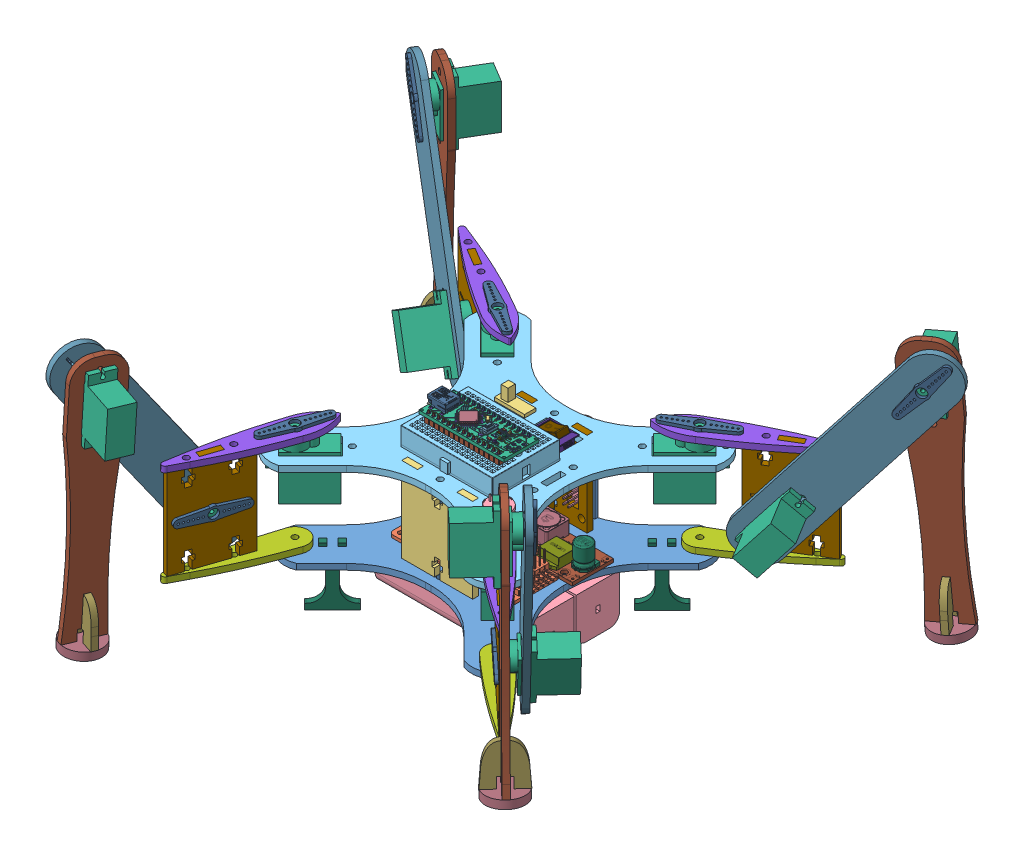
SolidWorks assembly SpiderBot_2_0, configuration Valor predeterminado. Lengths in mm.
Overall size (288.43 150.42 260.44).
147 component instances, 77 part files, 232 mates.
Components (placement in the parent):
- base-1: base [Valor predeterminado] at (7.4255 7.885 67) size (120.89 3 120.89)
- PCA9685-1: PCA9685 [Valor predeterminado] at (119.5232 12.385 80.9) size (67.25 16.5 25)
- suporte_mod-2: suporte_mod [Valor predeterminado] at (115.5232 50.885 96.5) size (36 46 3)
- Bateria-1: Bateria [Valor predeterminado] at (119.2732 7.885 80.5) x (-1 0 0) z (0 0 1) size (79 23 22)
- Bateria-3: Bateria [Valor predeterminado] at (119.2732 7.885 57.5) x (-1 0 0) z (0 0 1) size (79 23 22)
- Mini-Black.step-1: Mini-Black.step [Valor predeterminado] at (118.7863 59.6523 77.1335) size (48 9.4 35.7)
- Arduino_NANO_CH340.step-1: Arduino_NANO_CH340.step [Valor predeterminado] at (119.2913 68.1776 78.389) x (1 0 0) z (0 1 0) size (44.2 17.78 14.14)
  - Board_Geoms_6dc.step-1: Board_Geoms_6dc.step [Valor predeterminado] at origin size (44.2 17.78 2.36)
    - Pcb_6dc.step-1: Pcb_6dc.step [Valor predeterminado] at (-148.59 80.01 0) size (43.18 17.78 1.6)
    - topSilks_7595.step-1: topSilks_7595.step [Valor predeterminado] at (-148.59 80.01 0.07) size (44.2 13.15 0.15)
    - topTracks_6dc.step-1: topTracks_6dc.step [Valor predeterminado] at (-148.59 80.01 0.01) size (41.39 16.95 0.06)
    - botTracks_6dc.step-1: botTracks_6dc.step [Valor predeterminado] at (-148.59 80.01 -1.61) size (42.84 17.44 1.15)
  - Step_Models_6dc.step-1: Step_Models_6dc.step [Valor predeterminado] at origin size (41.36 17.78 14.14)
    - Top_6dc.step-1: Top_6dc.step [Valor predeterminado] at origin size (35.07 12.73 5)
      - J1_USB_Mini-B_Lumberg_2486_01_Horizontal_5F4AD4E6.step-1: J1_USB_Mini-B_Lumberg_2486_01_Horizontal_5F4AD4E6.step [Valor predeterminado] at (-16.51 0 0) x (0 -1 0) z (0 0 1) size (9.9 9.21 5)
      - R1_R_0603_1608Metric_5F4AD58B.step-1: R1_R_0603_1608Metric_5F4AD58B.step [Valor predeterminado] at (9.0425 3.81 0) size (1.6 0.8 0.45)
      - D1_LED_0603_1608Metric_5F4AD4A1.step-1: D1_LED_0603_1608Metric_5F4AD4A1.step [Valor predeterminado] at (11.9635 3.81 0) x (-1 0 0) z (0 0 1) size (1.6 0.8 1.1)
      - U1_TQFP_32_7x7mm_P08mm_5F4B89F1.step-1: U1_TQFP_32_7x7mm_P08mm_5F4B89F1.step [Valor predeterminado] at (-5.08 0 0) x (-0.707107 -0.707107 0) z (0 0 1) size (9 9 1.1)
      - SW1_SW_SPST_CK_RS282G05A3_5F4B980B.step-1: SW1_SW_SPST_CK_RS282G05A3_5F4B980B.step [Valor predeterminado] at (4.826 0.09 0) x (0 1 0) z (0 0 1) size (8 3.5 2.5)
      - D2_LED_0603_1608Metric_5F4BB16E.step-1: D2_LED_0603_1608Metric_5F4BB16E.step [Valor predeterminado] at (11.9635 1.27 0) x (-1 0 0) z (0 0 1) size (1.6 0.8 1.1)
      - D3_LED_0603_1608Metric_5F4BB181.step-1: D3_LED_0603_1608Metric_5F4BB181.step [Valor predeterminado] at (11.9635 -1.27 0) x (-1 0 0) z (0 0 1) size (1.6 0.8 1.1)
      - D4_LED_0603_1608Metric_5F4BB194.step-1: D4_LED_0603_1608Metric_5F4BB194.step [Valor predeterminado] at (11.9635 -3.81 0) x (-1 0 0) z (0 0 1) size (1.6 0.8 1.1)
      - R2_R_0603_1608Metric_5F4BB207.step-1: R2_R_0603_1608Metric_5F4BB207.step [Valor predeterminado] at (9.0425 1.27 0) size (1.6 0.8 0.45)
      - R3_R_0603_1608Metric_5F4BB218.step-1: R3_R_0603_1608Metric_5F4BB218.step [Valor predeterminado] at (9.0425 -1.27 0) size (1.6 0.8 0.45)
      - R4_R_0603_1608Metric_5F4BB229.step-1: R4_R_0603_1608Metric_5F4BB229.step [Valor predeterminado] at (9.0425 -3.81 0) size (1.6 0.8 0.45)
      - Y1_muRata_CSTxExxV_5F4BB25D.step-1: Y1_muRata_CSTxExxV_5F4BB25D.step [Valor predeterminado] at (0.254 4.318 0) x (0.707107 -0.707107 0) z (0 0 1) size (3.2 1.35 0.9)
    - Bot_6dc.step-1: Bot_6dc.step [Valor predeterminado] at origin size (39.62 17.78 11.54)
      - D5_D_0805_5F4AD4B4.step-1: D5_D_0805_5F4AD4B4.step [Valor predeterminado] at (-18.9715 3.556 -1.6) x (-1 0 0) z (0 0 -1) size (2 1.27 0.8)
      - U2_SOP_16_44x104mm_P127mm_5F4C8504.step-1: U2_SOP_16_44x104mm_P127mm_5F4C8504.step [Valor predeterminado] at (-9.53 0.356 -1.6) x (0 1 0) z (0 0 -1) size (6.4 10.4 2.1)
      - C1_C_0603_1608Metric_5F4BB0F2.step-1: C1_C_0603_1608Metric_5F4BB0F2.step [Valor predeterminado] at (-7.0865 -4.826 -1.6) x (-1 0 0) z (0 0 -1) size (1.6 0.8 0.8)
      - C2_C_0603_1608Metric_5F4BB0F3.step-1: C2_C_0603_1608Metric_5F4BB0F3.step [Valor predeterminado] at (-19.5325 -2.286 -1.6) x (-1 0 0) z (0 0 -1) size (1.6 0.8 0.8)
      - C4_C_0603_1608Metric_5F4BB124.step-1: C4_C_0603_1608Metric_5F4BB124.step [Valor predeterminado] at (9.1185 -4.064 -1.6) x (1 0 0) z (0 0 -1) size (1.6 0.8 0.8)
      - C5_C_0603_1608Metric_5F4BB135.step-1: C5_C_0603_1608Metric_5F4BB135.step [Valor predeterminado] at (10.6425 3.81 -1.6) x (1 0 0) z (0 0 -1) size (1.6 0.8 0.8)
      - J2_PinHeader_1x15_P254mm_Vertical_5F4BB1B7.step-1: J2_PinHeader_1x15_P254mm_Vertical_5F4BB1B7.step [Valor predeterminado] at (17.78 7.62 -1.6) x (0 1 0) z (0 0 -1) size (2.54 38.1 11.54)
      - J3_PinHeader_1x15_P254mm_Vertical_5F4BB1DA.step-1: J3_PinHeader_1x15_P254mm_Vertical_5F4BB1DA.step [Valor predeterminado] at (17.78 -7.62 -1.6) x (0 1 0) z (0 0 -1) size (2.54 38.1 11.54)
      - R5_R_0603_1608Metric_5F4BB23A.step-1: R5_R_0603_1608Metric_5F4BB23A.step [Valor predeterminado] at (-0.9905 -2.54 -1.6) x (-1 0 0) z (0 0 -1) size (1.6 0.8 0.45)
      - R6_R_0603_1608Metric_5F4BB24B.step-1: R6_R_0603_1608Metric_5F4BB24B.step [Valor predeterminado] at (-1.016 -4.318 -1.6) x (-1 0 0) z (0 0 -1) size (1.6 0.8 0.45)
      - R7_R_0603_1608Metric_5F4BB25C.step-1: R7_R_0603_1608Metric_5F4BB25C.step [Valor predeterminado] at (14.9605 3.81 -1.6) x (-1 0 0) z (0 0 -1) size (1.6 0.8 0.45)
      - Y2_muRata_CSTxExxV_5F4BB293.step-1: Y2_muRata_CSTxExxV_5F4BB293.step [Valor predeterminado] at (-13.462 -4.826 -1.6) x (-1 0 0) z (0 0 -1) size (3.2 1.35 0.9)
      - C6_CP_EIA_3216_18_Kemet_A_5F4BFB24.step-1: C6_CP_EIA_3216_18_Kemet_A_5F4BFB24.step [Valor predeterminado] at (-18.97 0 -1.6) x (-1 0 0) z (0 0 -1) size (3.2 1.6 1.8)
      - C7_CP_EIA_3216_18_Kemet_A_5F4BFB36.step-1: C7_CP_EIA_3216_18_Kemet_A_5F4BFB36.step [Valor predeterminado] at (12.62 1.27 -1.6) x (-1 0 0) z (0 0 -1) size (3.2 1.6 1.8)
      - U3_SOT_89_3_5F4BFB48.step-1: U3_SOT_89_3_5F4BFB48.step [Valor predeterminado] at (12.7 -2.54 -1.6) x (-1 0 0) z (0 0 -1) size (4 4.5 1.52)
- Camera OV7670.STEP-1: Camera OV7670.STEP [Valor predeterminado] at (119.0232 31.335 36.768) x (0 -1 0) z (0 0 -1) size (34 35 28.6)
  - PcbForCamera.STEP-1: PcbForCamera.STEP [Valor predeterminado] at origin size (34 35 1.5)
  - CameraLens.STEP-1: CameraLens.STEP [Valor predeterminado] at (0 4.5 1.5) size (24 17.5 18.5)
  - pan head cross recess screw_iso_ISO 7045 - M1.6 x 6 - Z - 6N.STEP-1: pan head cross recess screw_iso_ISO 7045 - M1.6 x 6 - Z - 6N.STEP [Valor predeterminado] at (-10 4.5 -1.3) x (0 0 1) z (-0.934163 -0.356846 0) size (7.27 3.2 3.2)
  - pan head cross recess screw_iso_ISO 7045 - M1.6 x 6 - Z - 6N.STEP-2: pan head cross recess screw_iso_ISO 7045 - M1.6 x 6 - Z - 6N.STEP [Valor predeterminado] at (10 4.5 -1.3) x (0 0 1) z (-0.934163 -0.356846 0) size (7.27 3.2 3.2)
  - PLS (DS1021-2xN)_DS1021-2x9.STEP-1: PLS (DS1021-2xN)_DS1021-2x9.STEP [Valor predeterminado] at (-10.16 -10.96 -2.5) size (22.86 5.08 11.6)
  - CAP 1206___ _________.STEP-1: CAP 1206___ _________.STEP [Valor predeterminado] at (12.3944 -3.3656 -0.812) size (3.2 1.62 1.62)
  - CAP 1206___ _________.STEP-2: CAP 1206___ _________.STEP [Valor predeterminado] at (8.833 13.1436 -0.812) size (3.2 1.62 1.62)
  - CAP 1206___ _________.STEP-3: CAP 1206___ _________.STEP [Valor predeterminado] at (-4.7413 13.3527 -0.812) size (3.2 1.62 1.62)
  - CAP 1206___ _________.STEP-4: CAP 1206___ _________.STEP [Valor predeterminado] at (-12.2243 8.8938 -0.812) size (3.2 1.62 1.62)
  - CAP 1206___ _________.STEP-5: CAP 1206___ _________.STEP [Valor predeterminado] at (-11.8299 -3.7667 -0.812) size (3.2 1.62 1.62)
  - CAP 0603___ _________.STEP-1: CAP 0603___ _________.STEP [Valor predeterminado] at (13.1952 -0.5568 -0.412) size (1.6 0.82 0.82)
  - CAP 0603___ _________.STEP-2: CAP 0603___ _________.STEP [Valor predeterminado] at (14.6505 6.2818 -0.412) size (1.6 0.82 0.82)
  - CAP 0603___ _________.STEP-3: CAP 0603___ _________.STEP [Valor predeterminado] at (8.112 11.3604 -0.412) size (1.6 0.82 0.82)
  - CAP 0603___ _________.STEP-4: CAP 0603___ _________.STEP [Valor predeterminado] at (-14.0856 5.7012 -0.412) size (1.6 0.82 0.82)
  - CAP 0603___ _________.STEP-5: CAP 0603___ _________.STEP [Valor predeterminado] at (-13.8777 -1.2547 -0.412) size (1.6 0.82 0.82)
  - CAP 0603___ _________.STEP-6: CAP 0603___ _________.STEP [Valor predeterminado] at (9.9936 -5.5766 -0.412) x (0 -1 0) z (0 0 1) size (1.6 0.82 0.82)
  - Stackpole CSR0402 Res___ _________.STEP-1: Stackpole CSR0402 Res___ _________.STEP [Valor predeterminado] at (2.2276 13.9111 0) x (0 -1 0) z (1 0 0) size (0.5 0.32 1.05)
  - Stackpole CSR0402 Res___ _________.STEP-2: Stackpole CSR0402 Res___ _________.STEP [Valor predeterminado] at (-9.8479 14.1877 0) x (0 -1 0) z (1 0 0) size (0.5 0.32 1.05)
  - SC-70-5___ _________.STEP-1: SC-70-5___ _________.STEP [Valor predeterminado] at (14.6025 3.5126 0) x (1 0 0) z (0 1 0) size (2 1.1 2.12)
  - SC-70-5___ _________.STEP-2: SC-70-5___ _________.STEP [Valor predeterminado] at (-14.2433 2.7104 0) x (-1 0 0) z (0 -1 0) size (2 1.1 2.12)
  - Stackpole CSR0402 Res___ _________.STEP-3: Stackpole CSR0402 Res___ _________.STEP [Valor predeterminado] at (-10.4133 -5.8042 0) x (-1 0 0) z (0 -1 0) size (0.5 0.32 1.05)
- suporte_mod_cam-1: suporte_mod_cam [Valor predeterminado] at (123.0232 10.885 38.5) x (-1 0 0) z (0 0 1) size (36 46 3)
- UBEC_certo-1: UBEC_certo [Valor predeterminado] at (100.2806 26.8872 90.152) size (44 18 7.45)
- LM2596 DC-DC StepDown Converter v1.step-1: LM2596 DC-DC StepDown Converter v1.step [Valor predeterminado] at (113.7732 22.2177 57.2327) x (-1 0 0) z (0 1 0) size (43 21 14.15)
  - Board v5.step-1: Board v5.step [Valor predeterminado] at (0 -9.7327 -11.3327) x (1 0 0) z (0 -1 0) size (43 1.7 21)
  - Trimpot 3296W v1.step-1: Trimpot 3296W v1.step [Valor predeterminado] at (-14.54 7.2723 -9.7327) x (-1 0 0) z (0 0 1) size (9.56 4.83 14.15)
  - CDRH127_470M v1.step-1: CDRH127_470M v1.step [Valor predeterminado] at (-15.855 -2.8827 -9.7427) x (0 -1 0) z (0 0 1) size (12.76 12.29 7.41)
  - CAPSMD220-35 v1.step-1: CAPSMD220-35 v1.step [Valor predeterminado] at (-4.2601 1.0246 -9.7327) x (0 1 0) z (0 0 1) size (9 8.3 10.7)
  - CAPSMD100-50 v1.step-1: CAPSMD100-50 v1.step [Valor predeterminado] at (-38.35 0.7473 -9.7327) x (0 1 0) z (0 0 1) size (9 8.3 10.7)
  - TO-263BA v2.step-1: TO-263BA v2.step [Valor predeterminado] at (-31.9 -3.4327 -9.7327) size (10.64 15.85 4.81)
  - DO-214AC-DIOM5127X23N v1.step-1: DO-214AC-DIOM5127X23N v1.step [Valor predeterminado] at (-32.735 -7.9827 -9.7327) size (5.3 2.8 2.3)
  - Resistor 0603 v1.step-1: Resistor 0603 v1.step [Valor predeterminado] at (-19.95 10.2673 -9.7327) x (0 -1 0) z (-1 0 0) size (2.1 0.6 0.8)
  - Resistor 0603 v1 (1).step-1: Resistor 0603 v1 (1).step [Valor predeterminado] at (-6.75 9.7673 -9.7327) x (0 -1 0) z (-1 0 0) size (2.1 0.6 0.8)
  - CAP0603 v1.step-1: CAP0603 v1.step [Valor predeterminado] at (-21.085 5.9823 -9.7327) x (0 -1 0) z (0 0 1) size (1.61 0.81 0.31)
  - FCrth 150060BS55040 v1.step-1: FCrth 150060BS55040 v1.step [Valor predeterminado] at (-5.89 8.9773 -9.7327) x (0 -1 0) z (0 0 1) size (1.6 0.8 0.4)
  - CAP0603 v1 (1).step-1: CAP0603 v1 (1).step [Valor predeterminado] at (-35.385 -5.5177 -9.7327) x (0 -1 0) z (0 0 1) size (1.61 0.81 0.31)
- base_cima-1: base_cima [Valor predeterminado] at (7.4255 50.885 67) size (128.99 3 128.99)
- Servo-1: Servo [Valor predeterminado] at (59.6659 32.485 17.5951) x (0.707107 0 0.707107) z (-0.707107 0 0.707107) size (31.9 29.9 11.8)
- Servo-2: Servo [Valor predeterminado] at (170.5367 32.485 9.2513) x (-0.707107 0 0.707107) z (-0.707107 0 -0.707107) size (31.9 29.9 11.8)
- Servo-3: Servo [Valor predeterminado] at (178.6684 32.485 119.9099) x (-0.707107 0 -0.707107) z (0.707107 0 -0.707107) size (31.9 29.9 11.8)
- Servo-4: Servo [Valor predeterminado] at (67.8684 32.485 128.6073) x (0.707107 0 -0.707107) z (0.707107 0 0.707107) size (31.9 29.9 11.8)
- Perna_baciadown-1: Perna_baciadown [Valor predeterminado] at (183.5595 10.885 132.1762) x (0.67976 0 -0.733435) z (0.733435 0 0.67976) size (13 3 60.1)
- Perna_baciaup-1: Perna_baciaup [Valor predeterminado] at (170.444 59.485 119.9618) x (0.67976 0 -0.733435) z (0.733435 0 0.67976) size (13.12 3 71.83)
- Perna_coxa-1: Perna_coxa [Valor predeterminado] at (196.281 36.385 141.9216) x (0 1 0) z (0.733435 0 0.67976) size (51.6 3 36)
- Servo_knob2-1: Servo_knob2 [Valor predeterminado] at (170.3246 59.185 119.9099) x (-0.727643 0 -0.685956) z (0.685956 0 -0.727643) size (32.4 4.8 6.6)
- Servo-6: Servo [Valor predeterminado] at (212.0513 44.249 119.7247) x (-0.251237 -0.9395 -0.232851) z (-0.689062 0.342549 -0.638634) size (31.9 29.9 11.8)
- Servo_knob2-3: Servo_knob2 [Valor predeterminado] at (196.4849 36.685 141.7016) x (0.733432 -0.00261 0.679757) z (-0.001914 -0.999997 -0.001774) size (32.4 4.8 6.6)
- Pé_com_antiderrapante-1: Pé_com_antiderrapante [Valor predeterminado] at (215.1821 130.5825 159.4395) x (0.729921 0.097767 0.676503) z (-0.67976 0 0.733435) size (24 122.6 3)
- comp_pé-1: comp_pé [Valor predeterminado] at (230.6854 6.2285 162.9006) x (-0.67976 0 0.733435) z (-0.729921 -0.097767 -0.676503) size (19 20 3)
- Antiderrapante-1: Antiderrapante [Valor predeterminado] at (223.4327 2.1038 169.1472) x (0.729921 0.097767 0.676503) z (-0.67976 0 0.733435) size (19 4 19)
- Canela_mod-1: Canela_mod [Valor predeterminado] at (219.7108 109.8107 156.0015) x (0.689062 -0.342549 0.638634) z (0.251237 0.9395 0.232851) size (24 3 124.6)
- Servo_knob2-4: Servo_knob2 [Valor predeterminado] at (220.1772 112.2805 156.8427) x (-0.247031 -0.941571 -0.228953) z (0.690581 -0.336814 0.640042) size (32.4 4.8 6.6)
- Servo-7: Servo [Valor predeterminado] at (205.9111 118.729 180.0247) x (0.071706 -0.995209 0.066458) z (0.729921 0.097767 0.676503) size (31.9 29.9 11.8)
- Perna_baciaup-2: Perna_baciaup [Valor predeterminado] at (67.8822 59.485 17.5691) x (-0.51295 0 0.858418) z (-0.858418 0 -0.51295) size (13.12 3 71.83)
- Servo_knob2-8: Servo_knob2 [Valor predeterminado] at (68.0098 59.185 17.5951) x (0.851179 0 0.524875) z (-0.524875 0 0.851179) size (32.4 4.8 6.6)
- Servo_knob2-9: Servo_knob2 [Valor predeterminado] at (-3.6674 103.1368 -17.3143) x (0.479294 -0.829608 0.286404) z (-0.712151 -0.558346 -0.425548) size (32.4 4.8 6.6)
- Servo-11: Servo [Valor predeterminado] at (4.9713 109.0457 -43.2559) x (-0.001293 -0.999999 -0.000773) z (-0.858417 0.001507 -0.51295) size (31.9 29.9 11.8)
- Pé_com_antiderrapante-3: Pé_com_antiderrapante [Valor predeterminado] at (-0.8391 121.5366 -21.7984) x (-0.858417 0.001507 -0.51295) z (0.51295 0 -0.858418) size (24 122.6 3)
- comp_pé-3: comp_pé [Valor predeterminado] at (-6.3922 -3.561 -15.7971) x (0.51295 0 -0.858418) z (0.858417 -0.001507 0.51295) size (19 20 3)
- Antiderrapante-3: Antiderrapante [Valor predeterminado] at (-0.2553 -7.5632 -23.2104) x (-0.858417 0.001507 -0.51295) z (0.51295 0 -0.858418) size (19 4 19)
- Canela_mod-3: Canela_mod [Valor predeterminado] at (-2.5388 100.9682 -16.2903) x (-0.709215 -0.563394 -0.423794) z (-0.483627 0.826189 -0.288993) size (24 3 124.6)
- Servo-12: Servo [Valor predeterminado] at (25.5355 44.8835 25.4151) x (0.483627 -0.826189 0.288993) z (0.709215 0.563394 0.423794) size (31.9 29.9 11.8)
- Servo_knob2-10: Servo_knob2 [Valor predeterminado] at (37.9003 36.685 1.7) x (-0.858415 -0.00261 -0.512949) z (0.00224 -0.999997 0.001339) size (32.4 4.8 6.6)
- Perna_baciadown-3: Perna_baciadown [Valor predeterminado] at (52.5195 10.885 8.3389) x (-0.51295 0 0.858418) z (-0.858418 0 -0.51295) size (13 3 60.1)
- Perna_coxa-3: Perna_coxa [Valor predeterminado] at (38.0541 36.385 1.4424) x (0 1 0) z (-0.858418 0 -0.51295) size (51.6 3 36)
- Perna_coxa-4: Perna_coxa [Valor predeterminado] at (58.5011 36.385 152.982) x (0 1 0) z (-0.317345 0 0.94831) size (51.6 3 36)
- Servo_knob2-11: Servo_knob2 [Valor predeterminado] at (55.3717 36.685 151.9348) x (-0.317345 0.000085 0.94831) z (0.000027 1 -0.000081) size (32.4 4.8 6.6)
- Servo_knob2-12: Servo_knob2 [Valor predeterminado] at (67.8684 59.185 120.2635) x (0.325377 0 -0.945584) z (0.945584 0 0.325377) size (32.4 4.8 6.6)
- Perna_baciaup-3: Perna_baciaup [Valor predeterminado] at (67.8703 59.485 120.3937) x (0.94831 0 0.317345) z (-0.317345 0 0.94831) size (13.12 3 71.83)
- Perna_baciadown-4: Perna_baciadown [Valor predeterminado] at (62.1418 10.885 137.3758) x (0.94831 0 0.317345) z (-0.317345 0 0.94831) size (13 3 60.1)
- Servo_knob2-13: Servo_knob2 [Valor predeterminado] at (36.2364 103.1908 193.3603) x (0.180723 -0.822001 -0.540049) z (0.260858 0.569485 -0.779512) size (32.4 4.8 6.6)
- Servo-13: Servo [Valor predeterminado] at (63.5241 108.7739 195.9531) x (-0.016613 -0.998629 0.049644) z (0.31691 -0.05235 -0.94701) size (31.9 29.9 11.8)
- Pé_com_antiderrapante-4: Pé_com_antiderrapante [Valor predeterminado] at (41.5364 121.5708 194.2235) x (0.31691 -0.05235 -0.94701) z (0.94831 0 0.317345) size (24 122.6 3)
- comp_pé-4: comp_pé [Valor predeterminado] at (32.3471 -3.4362 196.4746) x (0.94831 0 0.317345) z (-0.31691 0.05235 0.94701) size (19 20 3)
- Antiderrapante-4: Antiderrapante [Valor predeterminado] at (40.8343 -7.3537 201.0851) x (0.31691 -0.05235 -0.94701) z (0.94831 0 0.317345) size (19 4 19)
- Canela_mod-4: Canela_mod [Valor predeterminado] at (36.4203 101.0099 191.8654) x (0.261955 0.564463 -0.782791) z (-0.179129 0.825458 0.535286) size (24 3 124.6)
- Servo-14: Servo [Valor predeterminado] at (27.4494 38.2248 151.2383) x (0.179129 -0.825458 -0.535286) z (-0.261955 -0.564463 0.782791) size (31.9 29.9 11.8)
- Servo-16: Servo [Valor predeterminado] at (227.1986 104.6122 -40.1648) x (0.063997 -0.997191 -0.038929) z (-0.851949 -0.074907 0.518239) size (31.9 29.9 11.8)
- Servo-17: Servo [Valor predeterminado] at (221.4875 37.5346 19.9606) x (-0.539458 -0.775437 0.328151) z (0.662494 -0.631425 -0.402994) size (31.9 29.9 11.8)
- Canela_mod-6: Canela_mod [Valor predeterminado] at (245.2223 97.1208 -19.5256) x (-0.662494 0.631425 0.402994) z (0.539458 0.775437 -0.328151) size (24 3 124.6)
- comp_pé-6: comp_pé [Valor predeterminado] at (253.5176 -7.3343 -21.7624) x (-0.519699 0 -0.85435) z (0.851949 0.074907 -0.518239) size (19 20 3)
- Pé_com_antiderrapante-6: Pé_com_antiderrapante [Valor predeterminado] at (242.6319 117.5265 -24.5045) x (-0.851949 -0.074907 0.518239) z (-0.519699 0 -0.85435) size (24 122.6 3)
- Servo_knob2-17: Servo_knob2 [Valor predeterminado] at (200.52 36.685 1.4632) x (0.85435 0.000085 -0.519699) z (-0.000073 1 0.000044) size (32.4 4.8 6.6)
- Servo_knob2-18: Servo_knob2 [Valor predeterminado] at (246.4787 99.1708 -20.6409) x (-0.543487 -0.771572 0.330602) z (-0.659192 0.636142 0.400985) size (32.4 4.8 6.6)
- Servo_knob2-19: Servo_knob2 [Valor predeterminado] at (170.5367 59.185 17.5951) x (-0.858727 0 0.512434) z (-0.512434 0 -0.858727) size (32.4 4.8 6.6)
- Perna_baciadown-6: Perna_baciadown [Valor predeterminado] at (185.9535 10.885 8.2171) x (-0.519699 0 -0.85435) z (0.85435 0 -0.519699) size (13 3 60.1)
- Perna_baciaup-5: Perna_baciaup [Valor predeterminado] at (170.6193 59.485 17.4944) x (-0.519699 0 -0.85435) z (0.85435 0 -0.519699) size (13.12 3 71.83)
- Perna_coxa-6: Perna_coxa [Valor predeterminado] at (198.805 36.385 -1.3562) x (0 1 0) z (0.85435 0 -0.519699) size (51.6 3 36)
- suporte_embaixo-1: suporte_embaixo [Valor predeterminado] at (74.9476 7.885 22.6787) x (0.707107 0 0.707107) z (-0.707107 0 0.707107) size (20 29.5 3)
- suporte_embaixo-2: suporte_embaixo [Valor predeterminado] at (156.5279 7.885 29.7498) x (0.707107 0 -0.707107) z (0.707107 0 0.707107) size (20 29.5 3)
- suporte_embaixo-3: suporte_embaixo [Valor predeterminado] at (158.6492 7.885 106.1289) x (0.707107 0 0.707107) z (-0.707107 0 0.707107) size (20 29.5 3)
- suporte_embaixo-4: suporte_embaixo [Valor predeterminado] at (82.0186 7.885 108.2502) x (-0.707107 0 0.707107) z (-0.707107 0 -0.707107) size (20 29.5 3)
- Placa_GY521-1: Placa_GY521 [Predeterminado] at (118.6183 50.885 67.7208) x (0.007037 0 -0.999975) z (-0.999975 0 -0.007037) size (20.27 65.96 16.25)
- KCD1-11-2P-Off.step-1: KCD1-11-2P-Off.step [Valor predeterminado] at (128.815 54.751 49.6928) x (0 0 -1) z (1 0 0) size (10.5 19.01 15.2)
  - eBom-prt0.step-1: eBom-prt0.step [Valor predeterminado] at origin size (10.5 16.7 15.2)
  - eBom-prt1.step-1: eBom-prt1.step [Valor predeterminado] at (0 -0.9 0) x (1 0 0) z (0 0.228555 0.973531) size (7.4 7.35 10.6)
  - eBom-prt2.step-1: eBom-prt2.step [Valor predeterminado] at (0 -4.8504 0.3584) x (1 0 0) z (0 -0.285651 0.958334) size (5.24 1.4 9.6)
  - eBom-prt3.step-1: eBom-prt3.step [Valor predeterminado] at (0 0.1321 -0.2423) x (1 0 0) z (0 0.228555 0.973531) size (2.38 6.89 2.38)
- switch_pequeno-1: switch_pequeno [Valor predeterminado] at (98.5232 55.5004 49.8053) size (15.35 16.5 5.75)
- Buzzer_Active.stp-1: Buzzer_Active.stp [Valor predeterminado] at (145.1358 57.9073 98.5749) x (0.989214 0 -0.146479) z (0 -1 0) size (11.85 11.85 12.2)
- LED-1: LED [Default] at (88.3285 7.585 43.1958) x (0 0 -1) z (-1 0 0) size (5.5 35.6 6)
- LED-2: LED [Default] at (94.5547 7.585 43.1958) x (-0.444848 0 -0.895606) z (-0.895606 0 0.444848) size (5.5 35.6 6)
- Antiderrapante-7: Antiderrapante [Valor predeterminado] at (249.9458 -11.2257 -30.7055) x (-0.903442 -0.074462 0.422195) z (-0.423908 0.008151 -0.905669) size (19 4 19)
- Harness_1-SpiderBot_2_0-1: Harness_1-SpiderBot_2_0 [Valor predeterminado] at origin
Mates (geometry in assembly coordinates):
- Bloquear1: lock: unknown of Mini-Black.step-1; unknown of Arduino_NANO_CH340.step-1/Board_Geoms_6dc.step-1/Pcb_6dc.step-1
- Coincidente34: coincident anti-aligned: plane of base-1 through (7.4255 10.885 38.5) normal (0 0 1); plane of suporte_mod_cam-1 through (123.0232 10.885 38.5) normal (0 0 -1)
- Coincidente35: coincident anti-aligned: plane of base-1 through (101.2732 10.885 67) normal (1 0 0); plane of suporte_mod_cam-1 through (101.2732 8.885 41.5) normal (-1 0 0)
- Coincidente39: coincident anti-aligned: plane of base-1 through (7.4255 10.885 67) normal (0 1 0); plane of suporte_mod_cam-1 through (120.7732 10.885 41.5) normal (0 -1 0)
- Coincidente40: coincident anti-aligned: plane of base-1 through (137.2732 10.885 67) normal (-1 0 0); plane of suporte_mod-2 through (137.2732 52.885 99.5) normal (1 0 0)
- Coincidente41: coincident anti-aligned: plane of base-1 through (7.4255 10.885 96.5) normal (0 0 1); plane of suporte_mod-2 through (115.5232 50.885 96.5) normal (0 0 -1)
- Coincidente42: coincident anti-aligned: plane of base-1 through (7.4255 10.885 67) normal (0 1 0); plane of suporte_mod-2 through (120.7732 10.885 99.5) normal (0 -1 0)
- Paralelo3: parallel anti-aligned: plane of Camera OV7670.STEP-1/PcbForCamera.STEP-1 through (119.0232 31.335 36.768) normal (0 0 1); plane of suporte_mod_cam-1 through (123.0232 10.885 38.5) normal (0 0 -1)
- Concêntrico2: concentric anti-aligned: circle of Camera OV7670.STEP-1/PcbForCamera.STEP-1; circle of suporte_mod_cam-1
- Paralelo4: parallel aligned: plane of Camera OV7670.STEP-1/PcbForCamera.STEP-1 through (136.5232 14.335 35.268) normal (1 0 0); plane of suporte_mod_cam-1 through (137.2732 52.885 41.5) normal (1 0 0)
- Coincidente43: coincident anti-aligned: plane of suporte_mod_cam-1 through (123.0232 10.885 41.5) normal (0 0 1); plane of base_cima-1 through (7.4255 53.885 41.5) normal (0 0 -1)
- Coincidente44: coincident anti-aligned: plane of suporte_mod_cam-1 through (137.2732 52.885 41.5) normal (1 0 0); plane of base_cima-1 through (137.2732 53.885 67) normal (-1 0 0)
- Coincidente45: coincident anti-aligned: plane of suporte_mod_cam-1 through (120.7732 50.885 41.5) normal (0 1 0); plane of base_cima-1 through (7.4255 50.885 67) normal (0 -1 0)
- Coincidente46: coincident anti-aligned: plane of base_cima-1 through (66.592 53.885 7.8335) normal (-0.707107 0 0.707107); plane of Servo-1 through (83.9197 55.185 25.1612) normal (0.707107 0 -0.707107)
- Coincidente47: coincident anti-aligned: plane of base_cima-1 through (8.8433 53.885 68.4178) normal (0.707107 0 0.707107); plane of Servo-1 through (68.0098 55.185 9.2513) normal (-0.707107 0 -0.707107)
- Coincidente48: coincident anti-aligned: plane of base_cima-1 through (7.4255 50.885 67) normal (0 -1 0); plane of Servo-1 through (56.3425 50.885 14.2717) normal (0 1 0)
- Coincidente49: coincident anti-aligned: plane of base_cima-1 through (6.8433 53.885 67.5822) normal (0.707107 0 -0.707107); plane of Servo-4 through (59.5245 55.185 120.2635) normal (-0.707107 0 0.707107)
- Coincidente50: coincident anti-aligned: plane of base_cima-1 through (60.1067 53.885 119.6813) normal (0.707107 0 0.707107); plane of Servo-4 through (75.4344 55.185 104.3536) normal (-0.707107 0 -0.707107)
- Coincidente51: coincident anti-aligned: plane of base_cima-1 through (7.4255 50.885 67) normal (0 -1 0); plane of Servo-4 through (64.545 50.885 131.9307) normal (0 1 0)
- Coincidente54: coincident anti-aligned: plane of base_cima-1 through (7.4255 50.885 67) normal (0 -1 0); plane of Servo-3 through (181.9918 50.885 123.2333) normal (0 1 0)
- Coincidente55: coincident anti-aligned: plane of base_cima-1 through (66.592 53.885 7.8335) normal (-0.707107 0 0.707107); plane of Servo-3 through (178.6684 55.185 119.9099) normal (0.707107 0 -0.707107)
- Coincidente56: coincident anti-aligned: plane of base_cima-1 through (103.592 53.885 163.1665) normal (0.707107 0 0.707107); plane of Servo-3 through (162.7585 55.185 104) normal (-0.707107 0 -0.707107)
- Coincidente57: coincident anti-aligned: plane of base_cima-1 through (117.8555 53.885 -43.43) normal (-0.707107 0 0.707107); plane of Servo-2 through (178.8806 55.185 17.5951) normal (0.707107 0 -0.707107)
- Coincidente58: coincident anti-aligned: plane of base_cima-1 through (60.1067 53.885 119.6813) normal (0.707107 0 0.707107); plane of Servo-2 through (170.5367 55.185 9.2513) normal (-0.707107 0 -0.707107)
- Coincidente59: coincident anti-aligned: plane of base_cima-1 through (7.4255 50.885 67) normal (0 -1 0); plane of Servo-2 through (173.8601 50.885 5.9279) normal (0 1 0)
- Concêntrico3: concentric aligned: circle of Servo-3; circle of Servo_knob2-1
- Coincidente60: coincident anti-aligned: plane of Servo-3 through (168.1439 59.185 117.7293) normal (0 1 0); plane of Servo_knob2-1 through (170.3246 59.185 119.9099) normal (0 -1 0)
- Concêntrico4: concentric aligned: circle of Perna_baciaup-1; circle of Servo_knob2-1
- Coincidente61: coincident anti-aligned: plane of Perna_baciaup-1 through (356.2324 62.485 -83.3641) normal (0 1 0); plane of Servo_knob2-1 through (170.3246 62.485 119.9099) normal (0 -1 0)
- Bloquear2: lock: unknown of Perna_baciaup-1; unknown of Servo_knob2-1
- Coincidente62: coincident anti-aligned: plane of Perna_baciaup-1 through (192.6138 62.485 138.5228) normal (-0.67976 0 0.733435); plane of Perna_coxa-1 through (196.281 36.385 141.9216) normal (0.67976 0 -0.733435)
- Coincidente63: coincident anti-aligned: plane of Perna_baciadown-1 through (184.5791 13.885 131.0761) normal (-0.67976 0 0.733435); plane of Perna_coxa-1 through (196.281 36.385 141.9216) normal (0.67976 0 -0.733435)
- Coincidente64: coincident anti-aligned: plane of Perna_baciadown-1 through (198.9285 13.885 146.4205) normal (-0.733435 0 -0.67976); plane of Perna_coxa-1 through (197.9089 13.885 147.5207) normal (0.733435 0 0.67976)
- Coincidente65: coincident anti-aligned: plane of Perna_baciaup-1 through (191.5942 62.485 139.6229) normal (0.733435 0 0.67976); plane of Perna_coxa-1 through (190.5745 62.485 140.7231) normal (-0.733435 0 -0.67976)
- Coincidente66: coincident anti-aligned: plane of Perna_baciaup-1 through (356.2324 59.485 -83.3641) normal (0 -1 0); plane of Perna_coxa-1 through (186.1739 59.485 136.6445) normal (0 1 0)
- Coincidente67: coincident anti-aligned: plane of Perna_baciadown-1 through (183.5595 13.885 132.1762) normal (0 1 0); plane of Perna_coxa-1 through (202.3095 13.885 151.5992) normal (0 -1 0)
- Coincidente68: coincident anti-aligned: plane of Servo-6 through (195.7101 33.7876 140.9835) normal (-0.67976 0 0.733435); plane of Servo_knob2-3 through (196.4849 36.685 141.7016) normal (0.67976 0 -0.733435)
- Concêntrico5: concentric aligned: circle of Servo-6; circle of Servo_knob2-3
- Concêntrico6: concentric aligned: cylinder of Perna_coxa-1 through (194.2417 36.685 144.1219) axis (0.67976 0 -0.733435) radius 3.5; cylinder of Servo_knob2-3 through (193.2221 36.685 145.222) axis (0.67976 0 -0.733435) radius 3.3
- Coincidente69: coincident anti-aligned: plane of Perna_coxa-1 through (194.2417 36.385 144.1219) normal (-0.67976 0 0.733435); plane of Servo_knob2-3 through (194.2417 36.685 144.1219) normal (0.67976 0 -0.733435)
- Bloquear3: lock: unknown of Perna_coxa-1; unknown of Servo_knob2-3
- Coincidente71: coincident anti-aligned: plane of Pé_com_antiderrapante-1 through (-68.8447 1.5173 -103.8014) normal (0.67976 0 -0.733435); plane of comp_pé-1 through (222.3405 15.8873 166.074) normal (-0.67976 0 0.733435)
- Coincidente72: coincident anti-aligned: plane of Pé_com_antiderrapante-1 through (222.491 16.1806 170.3038) normal (-0.729921 -0.097767 -0.676503); plane of comp_pé-1 through (218.7242 23.3757 173.3283) normal (0.729921 0.097767 0.676503)
- Coincidente73: coincident anti-aligned: plane of Pé_com_antiderrapante-1 through (220.3013 15.8873 168.2743) normal (0.071706 -0.995209 0.066458); plane of comp_pé-1 through (222.3405 15.8873 166.074) normal (-0.071706 0.995209 -0.066458)
- Coincidente74: coincident anti-aligned: plane of Pé_com_antiderrapante-1 through (219.8322 5.7763 167.8396) normal (0.071706 -0.995209 0.066458); plane of Antiderrapante-1 through (223.1459 6.0846 168.8814) normal (-0.071706 0.995209 -0.066458)
- Bloquear4: lock: unknown of comp_pé-1; unknown of Antiderrapante-1
- Coincidente78: coincident anti-aligned: plane of Servo-6 through (190.968 23.1103 131.1345) normal (-0.251237 -0.9395 -0.232851); plane of Canela_mod-1 through (198.0166 21.0593 131.8045) normal (0.251237 0.9395 0.232851)
- Coincidente79: coincident anti-aligned: plane of Servo-6 through (196.6208 44.249 136.3737) normal (-0.689062 0.342549 -0.638634); plane of Canela_mod-1 through (217.6245 111.8617 149.9774) normal (0.689062 -0.342549 0.638634)
- Coincidente80: coincident anti-aligned: plane of Servo-6 through (200.7246 48.6647 134.3143) normal (-0.67976 0 0.733435); plane of Canela_mod-1 through (221.7501 109.8107 153.8011) normal (0.67976 0 -0.733435)
- Concêntrico7: concentric aligned: circle of Servo_knob2-4; circle of Servo-7
- Coincidente81: coincident anti-aligned: plane of Servo_knob2-4 through (220.1772 112.2805 156.8427) normal (-0.67976 0 0.733435); plane of Servo-7 through (220.3984 109.2113 157.0477) normal (0.67976 0 -0.733435)
- Concêntrico8: concentric aligned: cylinder of Canela_mod-1 through (222.4204 112.2805 154.4224) axis (-0.67976 0 0.733435) radius 3.5; cylinder of Servo_knob2-4 through (223.4401 112.2805 153.3222) axis (-0.67976 0 0.733435) radius 3.3
- Coincidente82: coincident anti-aligned: plane of Canela_mod-1 through (221.7501 109.8107 153.8011) normal (0.67976 0 -0.733435); plane of Servo_knob2-4 through (222.4204 112.2805 154.4224) normal (-0.67976 0 0.733435)
- Bloquear5: lock: unknown of Canela_mod-1; unknown of Servo_knob2-4
- Coincidente84: coincident anti-aligned: plane of Pé_com_antiderrapante-1 through (220.0321 96.3368 168.0248) normal (-0.729921 -0.097767 -0.676503); plane of Servo-7 through (221.3417 118.729 163.3757) normal (0.729921 0.097767 0.676503)
- Coincidente85: coincident anti-aligned: plane of Pé_com_antiderrapante-1 through (-70.884 1.5173 -101.6011) normal (-0.67976 0 0.733435); plane of Servo-7 through (218.0817 123.4065 166.2172) normal (0.67976 0 -0.733435)
- Coincidente86: coincident anti-aligned: plane of Pé_com_antiderrapante-1 through (220.0321 96.3368 168.0248) normal (-0.071706 0.995209 -0.066458); plane of Servo-7 through (222.955 96.3368 164.871) normal (0.071706 -0.995209 0.066458)
- Concêntrico9: concentric aligned: cylinder of Servo_knob2-7 through (307.736 161.8953 -85.1543) axis (0.507094 0 -0.861891) radius 3.3; cylinder of Perna_coxa-2 through (308.4967 161.8953 -86.4471) axis (0.507094 0 -0.861891) radius 3.5
- Concêntrico11: concentric aligned: circle of Servo-10; circle of Servo_knob2-7
